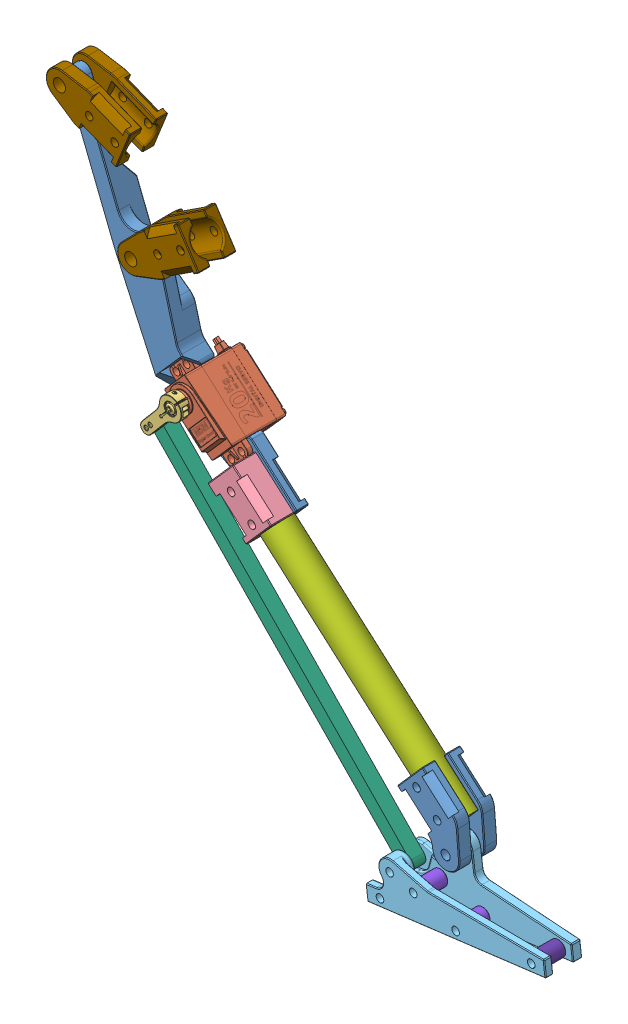
SolidWorks assembly Figuring out the legs, configuration Default. Lengths in mm.
Overall size (340.39 375.62 52.82).
16 component instances, 9 part files, 1 mates.
Components (placement in the parent):
- Sophia's Shin^Figuring out the legs-1: Sophia's Shin^Figuring out the legs [Default] at origin size (340.39 375.62 52.82) (virtual)
  - Shin_Upper^Sophia's Shin_Figuring out the legs-1: Shin_Upper^Sophia's Shin_Figuring out the legs [Default] at origin size (267.87 325.17 25) (virtual)
  - Servo^Sophia's Shin_Figuring out the legs-2: Servo^Sophia's Shin_Figuring out the legs [Default] at (30.2353 -67.9297 -4.25) x (0.660773 0.750586 0) z (0.750586 -0.660773 0) size (38.48 49.37 55.6) (virtual)
    - DS3218MG MS24 Digital Servo 270^Servo_Sophia's Shin_Figuring out the legs-1: DS3218MG MS24 Digital Servo 270^Servo_Sophia's Shin_Figuring out the legs [Default] at origin size (20.1 45.99 55.6) (virtual)
    - Servo Arm^Servo_Sophia's Shin_Figuring out the legs-1: Servo Arm^Servo_Sophia's Shin_Figuring out the legs [Default] x (-0.018595 0 -0.999827) z (0.999827 0 -0.018595) size (14.5 6.95 35.53) (virtual)
  - Shin Clamp^Sophia's Shin_Figuring out the legs-1: Shin Clamp^Sophia's Shin_Figuring out the legs [Default] at (58.5669 -92.8712 0) x (0 0 -1) z (-0.660773 -0.750586 0) size (15 33.83 25) (virtual)
  - Foot^Sophia's Shin_Figuring out the legs-1: Foot^Sophia's Shin_Figuring out the legs [Default] at (206.6131 -235.2675 0) x (0.992124 0.12526 0) z (0 0 1) size (118 46 24) (virtual)
  - Shin Linkage^Sophia's Shin_Figuring out the legs-1: Shin Linkage^Sophia's Shin_Figuring out the legs [Default] at (14.3911 -86.6169 1.75) x (0.697729 -0.716362 0) z (0 0 1) size (244 9 9) (virtual)
  - Shin Pipe^Sophia's Shin_Figuring out the legs-1: Shin Pipe^Sophia's Shin_Figuring out the legs [Default] at (205.4867 -222.2108 0) x (0.660773 0.750586 0) z (0 0 1) size (19.05 192 19.05) (virtual)
  - Foot Spacer^Sophia's Shin_Figuring out the legs-1: Foot Spacer^Sophia's Shin_Figuring out the legs [Default] at (172.0539 -272.8927 3) size (10 10 13) (virtual)
  - Foot Spacer^Sophia's Shin_Figuring out the legs-2: Foot Spacer^Sophia's Shin_Figuring out the legs [Default] at (193.8631 -258.9088 3) size (10 10 13) (virtual)
  - Foot Spacer^Sophia's Shin_Figuring out the legs-3: Foot Spacer^Sophia's Shin_Figuring out the legs [Default] at (271.2663 -260.3667 3) x (-0.993659 -0.112436 0) z (0 0 1) size (10 10 13) (virtual)
  - Foot Spacer^Sophia's Shin_Figuring out the legs-4: Foot Spacer^Sophia's Shin_Figuring out the legs [Default] at (271.2663 -260.3667 3) size (10 10 13) (virtual)
  - Foreleg-1: Foreleg [Default<As Machined>] at (251.2584 163.9183 0) x (-0.913132 -0.407664 0) z (0 0 -1) size (55.33 29.29 25)
  - Foreleg-2: Foreleg [Default<As Machined>] at (231.8854 -35.775 0) x (-0.858829 0.512263 0) z (0 0 -1) size (55.33 29.29 25)
  - Foot Spacer^Sophia's Shin_Figuring out the legs-5: Foot Spacer^Sophia's Shin_Figuring out the legs [Default] at (221.6601 -266.6297 3) x (0.906549 0.4221 0) z (0 0 1) size (10 10 13) (virtual)
Mates (geometry in assembly coordinates):
- Coincident1: coordinate: point of Sophia's Shin^David s assembly-1
